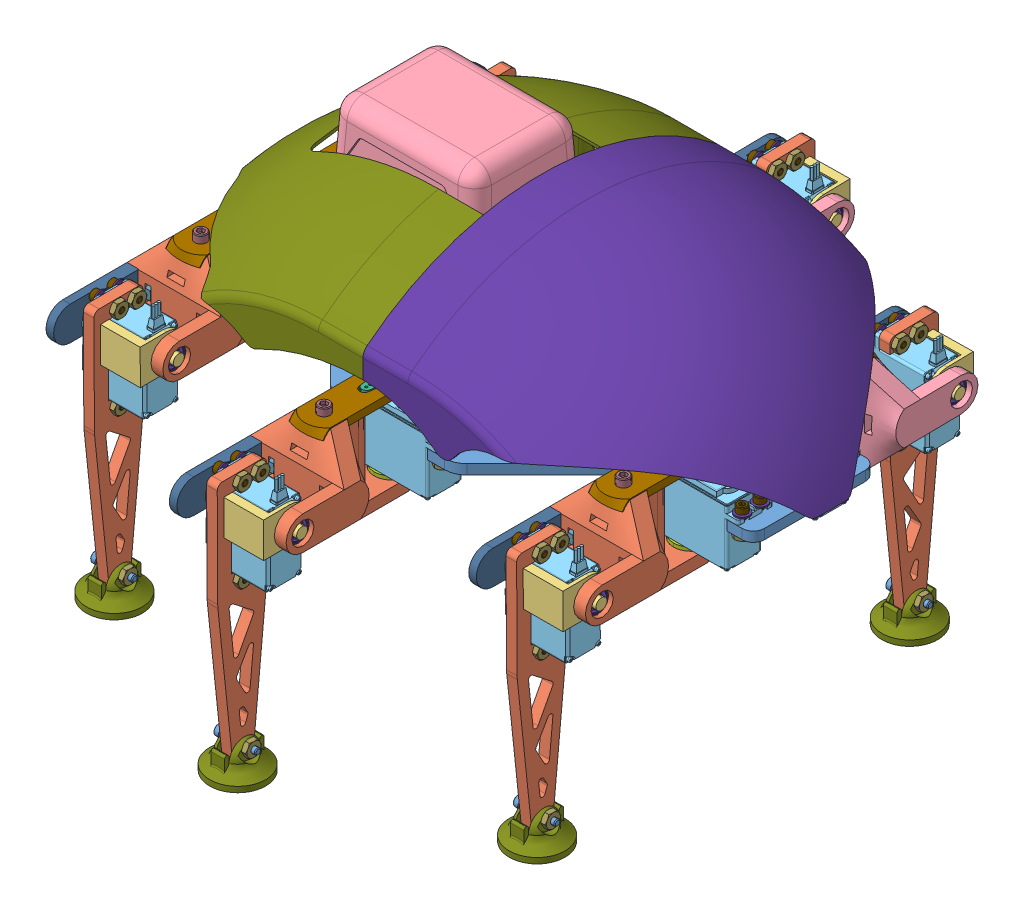
SolidWorks assembly Hexapod, configuration Défaut. Lengths in mm. (continued)
Components (placement in the parent): (continued)
- Leg_(Straight_Foot)_(Mirror)-5: Leg_(Straight_Foot)_(Mirror) [Default] at (-54.94 -26.67 49.906) size (70.36 162.3 124.8) (flexible) (continued)
  - HX-SHCS 0.138-32x0.5x0.5-N-15: HX-SHCS 0.138-32x0.5x0.5-N [HX-SHCS 0.138-32x0.5x0.5-N] at (-7.0087 -17.0352 62.351) x (0.999998 0 -0.002055) z (0.002055 0 0.999998) size (16.21 5.74 5.74)
  - HX-SHCS 0.138-32x0.5x0.5-N-16: HX-SHCS 0.138-32x0.5x0.5-N [HX-SHCS 0.138-32x0.5x0.5-N] at (-6.9874 30.4142 72.7445) x (0.999998 0 -0.002055) z (0.002055 0 0.999998) size (16.21 5.74 5.74)
  - HX-SHCS 0.138-32x0.5x0.5-N-17: HX-SHCS 0.138-32x0.5x0.5-N [HX-SHCS 0.138-32x0.5x0.5-N] at (-6.9878 -17.0852 72.5109) x (0.999998 0 -0.002055) z (0.002055 0 0.999998) size (16.21 5.74 5.74)
  - Narrow FW 0.138-8: Narrow FW 0.138 [Narrow FW 0.138] at (-3.81 29.1846 -4.826) x (0 -1 0) z (0.55878 0 -0.829316) size (0.81 7.92 7.92)
  - HX-SHCS 0.138-32x0.5x0.5-N-18: HX-SHCS 0.138-32x0.5x0.5-N [HX-SHCS 0.138-32x0.5x0.5-N] at (-3.81 33.7566 -4.826) x (0 -1 0) z (-0.55878 0 0.829316) size (16.21 5.74 5.74)
  - Narrow FW 0.138-9: Narrow FW 0.138 [Narrow FW 0.138] at (43.69 29.1846 -4.826) x (0 -1 0) z (0.55878 0 -0.829316) size (0.81 7.92 7.92)
  - Narrow FW 0.138-10: Narrow FW 0.138 [Narrow FW 0.138] at (-3.81 29.1846 -14.986) x (0 -1 0) z (0.55878 0 -0.829316) size (0.81 7.92 7.92)
  - Narrow FW 0.138-11: Narrow FW 0.138 [Narrow FW 0.138] at (43.69 29.1846 -14.986) x (0 -1 0) z (0.55878 0 -0.829316) size (0.81 7.92 7.92)
  - HX-SHCS 0.138-32x0.5x0.5-N-19: HX-SHCS 0.138-32x0.5x0.5-N [HX-SHCS 0.138-32x0.5x0.5-N] at (43.69 33.7566 -4.826) x (0 -1 0) z (-0.55878 0 0.829316) size (16.21 5.74 5.74)
  - HX-SHCS 0.138-32x0.5x0.5-N-20: HX-SHCS 0.138-32x0.5x0.5-N [HX-SHCS 0.138-32x0.5x0.5-N] at (-3.81 33.7566 -14.986) x (0 -1 0) z (-0.55878 0 0.829316) size (16.21 5.74 5.74)
  - HX-SHCS 0.138-32x0.5x0.5-N-21: HX-SHCS 0.138-32x0.5x0.5-N [HX-SHCS 0.138-32x0.5x0.5-N] at (43.69 33.7566 -14.986) x (0 -1 0) z (-0.55878 0 0.829316) size (16.21 5.74 5.74)
  - HX-SHCS 0.138-32x0.75x0.75-N-1: HX-SHCS 0.138-32x0.75x0.75-N [HX-SHCS 0.138-32x0.75x0.75-N] at (-7.8263 -99.7276 71.0261) x (0.999998 0 -0.002055) z (-0.001815 -0.46966 -0.882845) size (22.56 5.74 5.74)
  - Narrow FW 0.138-12: Narrow FW 0.138 [Narrow FW 0.138] at (-4.0671 -99.7276 71.0183) x (-0.999998 0 0.002055) z (-0.001688 -0.570502 -0.821294) size (0.81 7.92 7.92)
  - MSHXNUT 0.138-32-D-N-18: MSHXNUT 0.138-32-D-N [MSHXNUT 0.138-32-D-N] at (9.4457 -99.7276 70.9906) x (0 1 0) z (-0.999998 0 0.002055) size (7.92 9.15 2.9)
- Leg_(Straight_Foot)_(Mirror)-6: Leg_(Straight_Foot)_(Mirror) [Default] at (-174.94 -26.67 99.906) size (70.36 162.3 124.8) (flexible)
  - Joint_(Mirror)-1: Joint_(Mirror) [Défaut] at (36.4933 -51.1276 34.4889) x (0.002055 0 0.999998) z (0 -1 0) size (96.52 53.26 53.26)
  - hs-422-3: hs-422 [Défaut] at (19.939 20.701 -19.812) x (0 0 1) z (-1 0 0) size (19.81 42.09 58.23)
  - hs-422_horn_straight-2: hs-422_horn_straight [Default] at (9.652 42.5743 -9.906) x (0.002055 0 0.999998) z (0.999998 0 -0.002055) size (33.93 4.93 8.79)
  - Bearing_mount_leg-1: Bearing_mount_leg [Default] at (9.652 21 -22.406) x (0 0 -1) z (0 -1 0) size (35 20 30)
  - Bearing-1: Bearing [Default] at (9.652 -6.7498 -9.906) x (0.266287 0 0.963894) z (-0.963894 0 0.266287) size (13.87 4.75 13.87)
  - Joint_attachment_leg-1: Joint_attachment_leg [Défaut] at (-17.0066 26.5024 34.5989) x (0.002055 0 0.999998) z (0 1 0) size (74.32 19.07 4.32)
  - bearing_mount_foot-2: bearing_mount_foot [Default] at (6.7141 17.2663 79.9818) x (0.002055 -0.004919 0.999986) z (0.999998 0 -0.002055) size (25 20 29.5)
  - Bearing-3: Bearing [Default] at (29.1886 16.9774 67.524) x (-0.001098 -0.845349 -0.534213) z (0.001738 -0.534214 0.845347) size (13.87 4.75 13.87)
  - hs-422-4: hs-422 [Défaut] at (6.0779 6.6418 77.4268) x (-0.002055 0.004919 -0.999986) z (0.00001 0.999988 0.004919) size (19.81 42.09 58.23)
  - hs-422_horn_straight-3: hs-422_horn_straight [Default] at (-15.8156 16.9774 67.6165) x (-0.002055 0 -0.999998) z (0 -1 0) size (33.93 4.93 8.79)
  - Foot_(Straight)-2: Foot_(Straight) [Default] at (0.0967 4.6719 71.5233) x (-0.002055 0.004919 -0.999986) z (0.999998 0 -0.002055) size (28 145.4 6)
  - Joint_attachment_foot-2: Joint_attachment_foot [Défaut] at (36.4933 7.4524 34.4889) x (0.002055 0 0.999998) z (0 -1 0) size (64.08 6.7 19.07)
  - SBHCSCREW 0.138-32x0.25-HX-N-1: SBHCSCREW 0.138-32x0.25-HX-N [SBHCSCREW 0.138-32x0.25-HX-N] at (-19.1684 16.9774 67.6234) x (0.999998 0 -0.002055) z (0.002055 0 0.999998) size (8.2 6.65 6.65)
  - SBHCSCREW 0.138-32x0.25-HX-N-2: SBHCSCREW 0.138-32x0.25-HX-N [SBHCSCREW 0.138-32x0.25-HX-N] at (9.652 45.9271 -9.906) x (0 -1 0) z (-0.864996 0 0.501779) size (8.2 6.65 6.65)
  - HX-SHCS 0.112-40x0.5x0.5-N-5: HX-SHCS 0.112-40x0.5x0.5-N [HX-SHCS 0.112-40x0.5x0.5-N] at (-2.7306 21.6303 80.0227) x (0.999998 0 -0.002055) z (0.001019 -0.868474 0.495733) size (15.54 4.65 4.65)
  - HX-SHCS 0.112-40x0.5x0.5-N-6: HX-SHCS 0.112-40x0.5x0.5-N [HX-SHCS 0.112-40x0.5x0.5-N] at (-2.7307 11.6304 79.9735) x (0.999998 0 -0.002055) z (0.001036 0.863555 0.504253) size (15.54 4.65 4.65)
  - HX-SHCS 0.164-32x0.5x0.5-N-3: HX-SHCS 0.164-32x0.5x0.5-N [HX-SHCS 0.164-32x0.5x0.5-N] at (-21.1613 16.9774 39.9006) x (0.999998 0 -0.002055) z (0.001028 0.866025 0.499999) size (16.87 6.86 6.86)
  - HX-SHCS 0.164-32x0.5x0.5-N-4: HX-SHCS 0.164-32x0.5x0.5-N [HX-SHCS 0.164-32x0.5x0.5-N] at (9.7311 47.893 28.5918) x (0 -1 0) z (0.002055 0 0.999998) size (16.87 6.86 6.86)
  - MSHXNUT 0.138-32-D-N-14: MSHXNUT 0.138-32-D-N [MSHXNUT 0.138-32-D-N] at (6.0779 -17.0332 62.3241) x (-0.001785 -0.495734 -0.868473) z (-0.999998 0 0.002055) size (7.92 9.15 2.9)
  - MSHXNUT 0.138-32-D-N-15: MSHXNUT 0.138-32-D-N [MSHXNUT 0.138-32-D-N] at (8.9943 -17.0832 72.478) x (-0.001775 0.504254 -0.863554) z (0.999998 0 -0.002055) size (7.92 9.15 2.9)
  - MSHXNUT 0.138-32-D-N-16: MSHXNUT 0.138-32-D-N [MSHXNUT 0.138-32-D-N] at (8.9739 30.4662 62.5518) x (0.00001 0.999988 0.004919) z (0.999998 0 -0.002055) size (7.92 9.15 2.9)
  - MSHXNUT 0.138-32-D-N-17: MSHXNUT 0.138-32-D-N [MSHXNUT 0.138-32-D-N] at (6.0992 30.4162 72.7176) x (-0.001785 -0.495734 -0.868473) z (-0.999998 0 0.002055) size (7.92 9.15 2.9)
  - MSHXNUT 0.164-32-D-N-10: MSHXNUT 0.164-32-D-N [MSHXNUT 0.164-32-D-N] at (-6.4315 16.9774 39.8703) x (0.002055 0 0.999998) z (-0.999998 0 0.002055) size (8.74 10.09 3.3)
  - MSHXNUT 0.164-32-D-N-11: MSHXNUT 0.164-32-D-N [MSHXNUT 0.164-32-D-N] at (9.7311 29.8612 28.5918) x (-0.002055 0 -0.999998) z (0 -1 0) size (8.74 10.09 3.3)
  - Slipper-1: Slipper [Default] at (3.0957 -111.2276 71.0036) x (0.999998 0 -0.002055) z (0.002055 0 0.999998) size (35.48 18.25 37.71)
  - Narrow FW 0.138-4: Narrow FW 0.138 [Narrow FW 0.138] at (-2.4363 30.4642 62.5753) x (0.999998 0 -0.002055) z (0.002055 0 0.999998) size (0.81 7.92 7.92)
  - HX-SHCS 0.138-32x0.5x0.5-N-14: HX-SHCS 0.138-32x0.5x0.5-N [HX-SHCS 0.138-32x0.5x0.5-N] at (-7.0082 30.4642 62.5847) x (0.999998 0 -0.002055) z (0.002055 0 0.999998) size (16.21 5.74 5.74)
  - Narrow FW 0.138-5: Narrow FW 0.138 [Narrow FW 0.138] at (-2.4367 -17.0352 62.3416) x (0.999998 0 -0.002055) z (0.002055 0 0.999998) size (0.81 7.92 7.92)
  - Narrow FW 0.138-6: Narrow FW 0.138 [Narrow FW 0.138] at (-2.4154 30.4142 72.7351) x (0.999998 0 -0.002055) z (0.002055 0 0.999998) size (0.81 7.92 7.92)
  - Narrow FW 0.138-7: Narrow FW 0.138 [Narrow FW 0.138] at (-2.4158 -17.0852 72.5015) x (0.999998 0 -0.002055) z (0.002055 0 0.999998) size (0.81 7.92 7.92)
  - HX-SHCS 0.138-32x0.5x0.5-N-15: HX-SHCS 0.138-32x0.5x0.5-N [HX-SHCS 0.138-32x0.5x0.5-N] at (-7.0087 -17.0352 62.351) x (0.999998 0 -0.002055) z (0.002055 0 0.999998) size (16.21 5.74 5.74)
  - HX-SHCS 0.138-32x0.5x0.5-N-16: HX-SHCS 0.138-32x0.5x0.5-N [HX-SHCS 0.138-32x0.5x0.5-N] at (-6.9874 30.4142 72.7445) x (0.999998 0 -0.002055) z (0.002055 0 0.999998) size (16.21 5.74 5.74)
  - HX-SHCS 0.138-32x0.5x0.5-N-17: HX-SHCS 0.138-32x0.5x0.5-N [HX-SHCS 0.138-32x0.5x0.5-N] at (-6.9878 -17.0852 72.5109) x (0.999998 0 -0.002055) z (0.002055 0 0.999998) size (16.21 5.74 5.74)
  - Narrow FW 0.138-8: Narrow FW 0.138 [Narrow FW 0.138] at (-3.81 29.1846 -4.826) x (0 -1 0) z (0.55878 0 -0.829316) size (0.81 7.92 7.92)
  - HX-SHCS 0.138-32x0.5x0.5-N-18: HX-SHCS 0.138-32x0.5x0.5-N [HX-SHCS 0.138-32x0.5x0.5-N] at (-3.81 33.7566 -4.826) x (0 -1 0) z (-0.55878 0 0.829316) size (16.21 5.74 5.74)
  - Narrow FW 0.138-9: Narrow FW 0.138 [Narrow FW 0.138] at (43.69 29.1846 -4.826) x (0 -1 0) z (0.55878 0 -0.829316) size (0.81 7.92 7.92)
  - Narrow FW 0.138-10: Narrow FW 0.138 [Narrow FW 0.138] at (-3.81 29.1846 -14.986) x (0 -1 0) z (0.55878 0 -0.829316) size (0.81 7.92 7.92)
  - Narrow FW 0.138-11: Narrow FW 0.138 [Narrow FW 0.138] at (43.69 29.1846 -14.986) x (0 -1 0) z (0.55878 0 -0.829316) size (0.81 7.92 7.92)
  - HX-SHCS 0.138-32x0.5x0.5-N-19: HX-SHCS 0.138-32x0.5x0.5-N [HX-SHCS 0.138-32x0.5x0.5-N] at (43.69 33.7566 -4.826) x (0 -1 0) z (-0.55878 0 0.829316) size (16.21 5.74 5.74)
  - HX-SHCS 0.138-32x0.5x0.5-N-20: HX-SHCS 0.138-32x0.5x0.5-N [HX-SHCS 0.138-32x0.5x0.5-N] at (-3.81 33.7566 -14.986) x (0 -1 0) z (-0.55878 0 0.829316) size (16.21 5.74 5.74)
  - HX-SHCS 0.138-32x0.5x0.5-N-21: HX-SHCS 0.138-32x0.5x0.5-N [HX-SHCS 0.138-32x0.5x0.5-N] at (43.69 33.7566 -14.986) x (0 -1 0) z (-0.55878 0 0.829316) size (16.21 5.74 5.74)
  - HX-SHCS 0.138-32x0.75x0.75-N-1: HX-SHCS 0.138-32x0.75x0.75-N [HX-SHCS 0.138-32x0.75x0.75-N] at (-7.8263 -99.7276 71.0261) x (0.999998 0 -0.002055) z (-0.001815 -0.46966 -0.882845) size (22.56 5.74 5.74)
  - Narrow FW 0.138-12: Narrow FW 0.138 [Narrow FW 0.138] at (-4.0671 -99.7276 71.0183) x (-0.999998 0 0.002055) z (-0.001688 -0.570502 -0.821294) size (0.81 7.92 7.92)
  - MSHXNUT 0.138-32-D-N-18: MSHXNUT 0.138-32-D-N [MSHXNUT 0.138-32-D-N] at (9.4457 -99.7276 70.9906) x (0 1 0) z (-0.999998 0 0.002055) size (7.92 9.15 2.9)
- Battery-1: Battery [Défaut] at (-118.1821 62.8376 15.5603) x (0 0 -1) z (-1 0 0) size (64.47 74.3 85.78)
  - MAKITA 4.0AH-1: MAKITA 4.0AH [Défaut] at (0.5853 -29.7874 85.4436) size (64.47 57.15 85.78)
  - MAKITA 4.0AH MOBILE-1: MAKITA 4.0AH MOBILE [Défaut] at (0.5853 -39.3124 91.7936) size (45.84 26.68 66.29)
- arduinoMega-1: arduinoMega [Detailed] at (-199.11 -7.6 14.62) x (0 0 -1) z (-1 0 0) size (108.32 14.5 53.3)
- raspberryPi3B-1: raspberryPi3B [Detailed] at (-109 6.35 15) x (-1 0 0) z (0 1 0) size (87.05 58.5 19.5)
- 12Channel PWM-1: 12Channel PWM [Default] at (-145.6 -5.6 15) x (-1 0 0) z (0 0 1) size (25.4 7.55 66.7)
- DROK_090483.stp-1: DROK_090483.stp [Default] at (-77.5 -5.6 45) x (-1 0 0) z (0 -1 0) size (50.02 60 18.9)
- HX-SHCS 0.138-32x0.625x0.625-N-2: HX-SHCS 0.138-32x0.625x0.625-N [HX-SHCS 0.138-32x0.625x0.625-N] at (-40.288 3.5052 19.09) x (0 -1 0) z (1 0 0) size (19.38 5.74 5.74)
- HX-SHCS 0.138-32x0.625x0.625-N-3: HX-SHCS 0.138-32x0.625x0.625-N [HX-SHCS 0.138-32x0.625x0.625-N] at (-50.288 3.5052 19.09) x (0 -1 0) z (0.5 0 0.866025) size (19.38 5.74 5.74)
- HX-SHCS 0.138-32x0.625x0.625-N-4: HX-SHCS 0.138-32x0.625x0.625-N [HX-SHCS 0.138-32x0.625x0.625-N] at (-50.288 3.5052 10.91) x (0 -1 0) z (1 0 0) size (19.38 5.74 5.74)
- HX-SHCS 0.138-32x0.625x0.625-N-5: HX-SHCS 0.138-32x0.625x0.625-N [HX-SHCS 0.138-32x0.625x0.625-N] at (-40.288 3.5052 10.91) x (0 -1 0) z (1 0 0) size (19.38 5.74 5.74)
- HX-SHCS 0.138-32x0.625x0.625-N-6: HX-SHCS 0.138-32x0.625x0.625-N [HX-SHCS 0.138-32x0.625x0.625-N] at (-170.288 3.5052 69.09) x (0 -1 0) z (1 0 0) size (19.38 5.74 5.74)
- HX-SHCS 0.138-32x0.625x0.625-N-7: HX-SHCS 0.138-32x0.625x0.625-N [HX-SHCS 0.138-32x0.625x0.625-N] at (-160.288 3.5052 69.09) x (0 -1 0) z (1 0 0) size (19.38 5.74 5.74)
- HX-SHCS 0.138-32x0.625x0.625-N-14: HX-SHCS 0.138-32x0.625x0.625-N [HX-SHCS 0.138-32x0.625x0.625-N] at (-160.288 3.5052 -39.09) x (0 -1 0) z (1 0 0) size (19.38 5.74 5.74)
- HX-SHCS 0.138-32x0.625x0.625-N-15: HX-SHCS 0.138-32x0.625x0.625-N [HX-SHCS 0.138-32x0.625x0.625-N] at (-170.288 3.5052 -39.09) x (0 -1 0) z (1 0 0) size (19.38 5.74 5.74)
- HX-SHCS 0.138-32x0.625x0.625-N-16: HX-SHCS 0.138-32x0.625x0.625-N [HX-SHCS 0.138-32x0.625x0.625-N] at (-280.288 3.5052 19.09) x (0 -1 0) z (1 0 0) size (19.38 5.74 5.74)
- HX-SHCS 0.138-32x0.625x0.625-N-17: HX-SHCS 0.138-32x0.625x0.625-N [HX-SHCS 0.138-32x0.625x0.625-N] at (-290.288 3.5052 19.09) x (0 -1 0) z (0.5 0 0.866025) size (19.38 5.74 5.74)
- HX-SHCS 0.138-32x0.625x0.625-N-18: HX-SHCS 0.138-32x0.625x0.625-N [HX-SHCS 0.138-32x0.625x0.625-N] at (-290.288 3.5052 10.91) x (0 -1 0) z (1 0 0) size (19.38 5.74 5.74)
- HX-SHCS 0.138-32x0.625x0.625-N-19: HX-SHCS 0.138-32x0.625x0.625-N [HX-SHCS 0.138-32x0.625x0.625-N] at (-280.288 3.5052 10.91) x (0 -1 0) z (1 0 0) size (19.38 5.74 5.74)
- MSHXNUT 0.138-32-D-N-60: MSHXNUT 0.138-32-D-N [MSHXNUT 0.138-32-D-N] at (-298.75 -8.4956 -15.08) x (1 0 0) z (0 -1 0) size (7.92 9.15 2.9)
- MSHXNUT 0.138-32-D-N-65: MSHXNUT 0.138-32-D-N [MSHXNUT 0.138-32-D-N] at (-298.75 -8.4956 -4.92) x (1 0 0) z (0 -1 0) size (7.92 9.15 2.9)
- MSHXNUT 0.138-32-D-N-70: MSHXNUT 0.138-32-D-N [MSHXNUT 0.138-32-D-N] at (-251.252 -8.4956 -4.92) x (0.5 0 0.866025) z (0 -1 0) size (7.92 9.15 2.9)
- MSHXNUT 0.138-32-D-N-75: MSHXNUT 0.138-32-D-N [MSHXNUT 0.138-32-D-N] at (-251.252 -8.4956 -15.08) x (0.5 0 0.866025) z (0 -1 0) size (7.92 9.15 2.9)
- MSHXNUT 0.138-32-D-N-80: MSHXNUT 0.138-32-D-N [MSHXNUT 0.138-32-D-N] at (-280.288 -13.5656 10.91) x (0 0 1) z (0 -1 0) size (7.92 9.15 2.9)
- MSHXNUT 0.138-32-D-N-85: MSHXNUT 0.138-32-D-N [MSHXNUT 0.138-32-D-N] at (-290.288 -13.5656 10.91) x (0 0 1) z (0 -1 0) size (7.92 9.15 2.9)
- MSHXNUT 0.138-32-D-N-88: MSHXNUT 0.138-32-D-N [MSHXNUT 0.138-32-D-N] at (-178.75 -8.4956 -65.08) x (1 0 0) z (0 -1 0) size (7.92 9.15 2.9)
- MSHXNUT 0.138-32-D-N-89: MSHXNUT 0.138-32-D-N [MSHXNUT 0.138-32-D-N] at (-178.75 -8.4956 -54.92) x (1 0 0) z (0 -1 0) size (7.92 9.15 2.9)
- MSHXNUT 0.138-32-D-N-90: MSHXNUT 0.138-32-D-N [MSHXNUT 0.138-32-D-N] at (-131.252 -8.4956 -54.92) x (0.5 0 0.866025) z (0 -1 0) size (7.92 9.15 2.9)
- MSHXNUT 0.138-32-D-N-91: MSHXNUT 0.138-32-D-N [MSHXNUT 0.138-32-D-N] at (-131.252 -8.4956 -65.08) x (0.5 0 0.866025) z (0 -1 0) size (7.92 9.15 2.9)
- MSHXNUT 0.138-32-D-N-92: MSHXNUT 0.138-32-D-N [MSHXNUT 0.138-32-D-N] at (-160.288 -13.5656 -39.09) x (0 0 1) z (0 -1 0) size (7.92 9.15 2.9)
- MSHXNUT 0.138-32-D-N-93: MSHXNUT 0.138-32-D-N [MSHXNUT 0.138-32-D-N] at (-170.288 -13.5656 -39.09) x (0 0 1) z (0 -1 0) size (7.92 9.15 2.9)
- MSHXNUT 0.138-32-D-N-94: MSHXNUT 0.138-32-D-N [MSHXNUT 0.138-32-D-N] at (-50.288 -13.5656 10.91) x (0 0 1) z (0 -1 0) size (7.92 9.15 2.9)
- MSHXNUT 0.138-32-D-N-95: MSHXNUT 0.138-32-D-N [MSHXNUT 0.138-32-D-N] at (-40.288 -13.5656 10.91) x (0 0 1) z (0 -1 0) size (7.92 9.15 2.9)
- MSHXNUT 0.138-32-D-N-96: MSHXNUT 0.138-32-D-N [MSHXNUT 0.138-32-D-N] at (-11.252 -8.4956 -4.92) x (0.5 0 0.866025) z (0 -1 0) size (7.92 9.15 2.9)
- MSHXNUT 0.138-32-D-N-97: MSHXNUT 0.138-32-D-N [MSHXNUT 0.138-32-D-N] at (-11.252 -8.4956 -15.08) x (0.5 0 0.866025) z (0 -1 0) size (7.92 9.15 2.9)
- MSHXNUT 0.138-32-D-N-98: MSHXNUT 0.138-32-D-N [MSHXNUT 0.138-32-D-N] at (-58.75 -8.4956 -4.92) x (1 0 0) z (0 -1 0) size (7.92 9.15 2.9)
- MSHXNUT 0.138-32-D-N-99: MSHXNUT 0.138-32-D-N [MSHXNUT 0.138-32-D-N] at (-58.75 -8.4956 -15.08) x (1 0 0) z (0 -1 0) size (7.92 9.15 2.9)
- MSHXNUT 0.138-32-D-N-100: MSHXNUT 0.138-32-D-N [MSHXNUT 0.138-32-D-N] at (-290.288 -10.67 19.09) x (0 0 -1) z (0 1 0) size (7.92 9.15 2.9)
- MSHXNUT 0.138-32-D-N-101: MSHXNUT 0.138-32-D-N [MSHXNUT 0.138-32-D-N] at (-280.288 -10.67 19.09) x (0 0 -1) z (0 1 0) size (7.92 9.15 2.9)
- MSHXNUT 0.138-32-D-N-102: MSHXNUT 0.138-32-D-N [MSHXNUT 0.138-32-D-N] at (-251.252 -5.6 34.92) x (0.5 0 -0.866025) z (0 1 0) size (7.92 9.15 2.9)
- MSHXNUT 0.138-32-D-N-103: MSHXNUT 0.138-32-D-N [MSHXNUT 0.138-32-D-N] at (-251.252 -5.6 45.08) x (0.5 0 -0.866025) z (0 1 0) size (7.92 9.15 2.9)
- MSHXNUT 0.138-32-D-N-104: MSHXNUT 0.138-32-D-N [MSHXNUT 0.138-32-D-N] at (-298.75 -5.6 34.92) x (1 0 0) z (0 1 0) size (7.92 9.15 2.9)
- MSHXNUT 0.138-32-D-N-105: MSHXNUT 0.138-32-D-N [MSHXNUT 0.138-32-D-N] at (-298.75 -5.6 45.08) x (1 0 0) z (0 1 0) size (7.92 9.15 2.9)
- MSHXNUT 0.138-32-D-N-106: MSHXNUT 0.138-32-D-N [MSHXNUT 0.138-32-D-N] at (-178.75 -5.6 95.08) x (1 0 0) z (0 1 0) size (7.92 9.15 2.9)
- MSHXNUT 0.138-32-D-N-107: MSHXNUT 0.138-32-D-N [MSHXNUT 0.138-32-D-N] at (-178.75 -5.6 84.92) x (1 0 0) z (0 1 0) size (7.92 9.15 2.9)
- MSHXNUT 0.138-32-D-N-108: MSHXNUT 0.138-32-D-N [MSHXNUT 0.138-32-D-N] at (-131.252 -5.6 84.92) x (0.5 0 -0.866025) z (0 1 0) size (7.92 9.15 2.9)
- MSHXNUT 0.138-32-D-N-109: MSHXNUT 0.138-32-D-N [MSHXNUT 0.138-32-D-N] at (-131.252 -5.6 95.08) x (0.5 0 -0.866025) z (0 1 0) size (7.92 9.15 2.9)
- MSHXNUT 0.138-32-D-N-110: MSHXNUT 0.138-32-D-N [MSHXNUT 0.138-32-D-N] at (-160.288 -10.67 69.09) x (0 0 -1) z (0 1 0) size (7.92 9.15 2.9)
- MSHXNUT 0.138-32-D-N-111: MSHXNUT 0.138-32-D-N [MSHXNUT 0.138-32-D-N] at (-170.288 -10.67 69.09) x (0 0 -1) z (0 1 0) size (7.92 9.15 2.9)
- MSHXNUT 0.138-32-D-N-112: MSHXNUT 0.138-32-D-N [MSHXNUT 0.138-32-D-N] at (-50.288 -10.67 19.09) x (0 0 -1) z (0 1 0) size (7.92 9.15 2.9)
- MSHXNUT 0.138-32-D-N-113: MSHXNUT 0.138-32-D-N [MSHXNUT 0.138-32-D-N] at (-40.288 -10.67 19.09) x (0 0 -1) z (0 1 0) size (7.92 9.15 2.9)
- MSHXNUT 0.138-32-D-N-114: MSHXNUT 0.138-32-D-N [MSHXNUT 0.138-32-D-N] at (-11.252 -5.6 34.92) x (0.5 0 -0.866025) z (0 1 0) size (7.92 9.15 2.9)
- MSHXNUT 0.138-32-D-N-115: MSHXNUT 0.138-32-D-N [MSHXNUT 0.138-32-D-N] at (-11.252 -5.6 45.08) x (0.5 0 -0.866025) z (0 1 0) size (7.92 9.15 2.9)
- MSHXNUT 0.138-32-D-N-116: MSHXNUT 0.138-32-D-N [MSHXNUT 0.138-32-D-N] at (-58.75 -5.6 34.92) x (1 0 0) z (0 1 0) size (7.92 9.15 2.9)
- MSHXNUT 0.138-32-D-N-117: MSHXNUT 0.138-32-D-N [MSHXNUT 0.138-32-D-N] at (-58.75 -5.6 45.08) x (1 0 0) z (0 1 0) size (7.92 9.15 2.9)
- HX-SHCS 0.138-32x0.5x0.5-N-20: HX-SHCS 0.138-32x0.5x0.5-N [HX-SHCS 0.138-32x0.5x0.5-N] at (-175 -12.6052 48.88) x (0 1 0) z (-0.5 0 -0.866025) size (16.21 5.74 5.74)
- HX-SHCS 0.138-32x0.5x0.5-N-21: HX-SHCS 0.138-32x0.5x0.5-N [HX-SHCS 0.138-32x0.5x0.5-N] at (-223.22 -12.6052 -32.36) x (0 1 0) z (1 0 0) size (16.21 5.74 5.74)
- HX-SHCS 0.138-32x0.5x0.5-N-22: HX-SHCS 0.138-32x0.5x0.5-N [HX-SHCS 0.138-32x0.5x0.5-N] at (-175 -12.6052 -26) x (0 1 0) z (-0.5 0 -0.866025) size (16.21 5.74 5.74)
- HX-SHCS 0.138-32x0.5x0.5-N-23: HX-SHCS 0.138-32x0.5x0.5-N [HX-SHCS 0.138-32x0.5x0.5-N] at (-223.22 -12.6052 50.11) x (0 1 0) z (-1 0 0) size (16.21 5.74 5.74)
- MSHXNUT 0.112-40-D-N-106: MSHXNUT 0.112-40-D-N [MSHXNUT 0.112-40-D-N] at (-223.22 2.4892 -32.36) x (1 0 0) z (0 1 0) size (6.35 7.33 2.49)
- MSHXNUT 0.112-40-D-N-107: MSHXNUT 0.112-40-D-N [MSHXNUT 0.112-40-D-N] at (-223.22 2.4892 50.11) x (1 0 0) z (0 1 0) size (6.35 7.33 2.49)
- MSHXNUT 0.112-40-D-N-108: MSHXNUT 0.112-40-D-N [MSHXNUT 0.112-40-D-N] at (-175 2.4892 -26) x (1 0 0) z (0 1 0) size (6.35 7.33 2.49)
- MSHXNUT 0.112-40-D-N-109: MSHXNUT 0.112-40-D-N [MSHXNUT 0.112-40-D-N] at (-175 2.4892 48.88) x (1 0 0) z (0 1 0) size (6.35 7.33 2.49)
- HX-SHCS 0.138-32x0.5x0.5-N-24: HX-SHCS 0.138-32x0.5x0.5-N [HX-SHCS 0.138-32x0.5x0.5-N] at (-117.315 -10.3052 -11.415) x (0 1 0) z (-0.5 0 -0.866025) size (16.21 5.74 5.74)
- MSHXNUT 0.112-40-D-N-110: MSHXNUT 0.112-40-D-N [MSHXNUT 0.112-40-D-N] at (-117.315 2.4892 -11.415) x (1 0 0) z (0 1 0) size (6.35 7.33 2.49)
- HX-SHCS 0.138-32x0.5x0.5-N-28: HX-SHCS 0.138-32x0.5x0.5-N [HX-SHCS 0.138-32x0.5x0.5-N] at (-80.685 -10.3052 -11.415) x (0 1 0) z (-0.5 0 -0.866025) size (16.21 5.74 5.74)
- HX-SHCS 0.138-32x0.5x0.5-N-29: HX-SHCS 0.138-32x0.5x0.5-N [HX-SHCS 0.138-32x0.5x0.5-N] at (-117.315 -10.3052 41.415) x (0 1 0) z (-0.5 0 -0.866025) size (16.21 5.74 5.74)
- HX-SHCS 0.138-32x0.5x0.5-N-30: HX-SHCS 0.138-32x0.5x0.5-N [HX-SHCS 0.138-32x0.5x0.5-N] at (-80.685 -10.3052 41.415) x (0 1 0) z (-0.5 0 -0.866025) size (16.21 5.74 5.74)
- MSHXNUT 0.112-40-D-N-114: MSHXNUT 0.112-40-D-N [MSHXNUT 0.112-40-D-N] at (-80.685 2.4892 -11.415) x (1 0 0) z (0 1 0) size (6.35 7.33 2.49)
- MSHXNUT 0.112-40-D-N-115: MSHXNUT 0.112-40-D-N [MSHXNUT 0.112-40-D-N] at (-117.315 2.4892 41.415) x (1 0 0) z (0 1 0) size (6.35 7.33 2.49)
- MSHXNUT 0.112-40-D-N-116: MSHXNUT 0.112-40-D-N [MSHXNUT 0.112-40-D-N] at (-80.685 2.4892 41.415) x (1 0 0) z (0 1 0) size (6.35 7.33 2.49)
- 1_4_Round_Aluminum_Standoff.step-1: 1_4_Round_Aluminum_Standoff.step [Défaut] at (-70 0 -9.5) x (0.963282 0 -0.268492) z (0.268492 0 0.963282) size (6.34 6.36 6.34)
- HX-SHCS 0.112-40x0.75x0.75-N-65: HX-SHCS 0.112-40x0.75x0.75-N [HX-SHCS 0.112-40x0.75x0.75-N] at (-70 10.4948 -9.5) x (0 -1 0) z (0.637638 0 0.770336) size (21.89 4.65 4.65)
- MSHXNUT 0.112-40-D-N-117: MSHXNUT 0.112-40-D-N [MSHXNUT 0.112-40-D-N] at (-70 -8.0892 -9.5) x (1 0 0) z (0 -1 0) size (6.35 7.33 2.49)
- 1_4_Round_Aluminum_Standoff.step-2: 1_4_Round_Aluminum_Standoff.step [Défaut] at (-128 0 -9.5) x (0.963282 0 -0.268492) z (0.268492 0 0.963282) size (6.34 6.36 6.34)
- 1_4_Round_Aluminum_Standoff.step-3: 1_4_Round_Aluminum_Standoff.step [Défaut] at (-70 0 39.5) x (0.963282 0 -0.268492) z (0.268492 0 0.963282) size (6.34 6.36 6.34)
- 1_4_Round_Aluminum_Standoff.step-4: 1_4_Round_Aluminum_Standoff.step [Défaut] at (-128 0 39.5) x (0.963282 0 -0.268492) z (0.268492 0 0.963282) size (6.34 6.36 6.34)
- MSHXNUT 0.112-40-D-N-121: MSHXNUT 0.112-40-D-N [MSHXNUT 0.112-40-D-N] at (-128 -8.0892 -9.5) x (1 0 0) z (0 -1 0) size (6.35 7.33 2.49)
- MSHXNUT 0.112-40-D-N-122: MSHXNUT 0.112-40-D-N [MSHXNUT 0.112-40-D-N] at (-70 -8.0892 39.5) x (1 0 0) z (0 -1 0) size (6.35 7.33 2.49)
- MSHXNUT 0.112-40-D-N-123: MSHXNUT 0.112-40-D-N [MSHXNUT 0.112-40-D-N] at (-128 -8.0892 39.5) x (1 0 0) z (0 -1 0) size (6.35 7.33 2.49)
- HX-SHCS 0.112-40x0.75x0.75-N-72: HX-SHCS 0.112-40x0.75x0.75-N [PreviewCfg] at (-128 10.4948 -9.5) x (0 -1 0) z (0.637638 0 0.770336) size (28.24 4.65 4.65)
- HX-SHCS 0.112-40x0.75x0.75-N-70: HX-SHCS 0.112-40x0.75x0.75-N [PreviewCfg] at (-70 10.4948 39.5) x (0 -1 0) z (0.637638 0 0.770336) size (28.24 4.65 4.65)
- HX-SHCS 0.112-40x0.75x0.75-N-71: HX-SHCS 0.112-40x0.75x0.75-N [PreviewCfg] at (-128 10.4948 39.5) x (0 -1 0) z (0.637638 0 0.770336) size (28.24 4.65 4.65)
- HX-SHCS 0.112-40x0.5x0.5-N-32: HX-SHCS 0.112-40x0.5x0.5-N [HX-SHCS 0.112-40x0.5x0.5-N] at (-155 -9.9448 -12.95) x (0 1 0) z (-1 0 0) size (15.54 4.65 4.65)
- MSHXNUT 0.112-40-D-N-124: MSHXNUT 0.112-40-D-N [MSHXNUT 0.112-40-D-N] at (-155 2.4892 -12.95) x (1 0 0) z (0 1 0) size (6.35 7.33 2.49)
- HX-SHCS 0.112-40x0.5x0.5-N-36: HX-SHCS 0.112-40x0.5x0.5-N [HX-SHCS 0.112-40x0.5x0.5-N] at (-136.2 -9.9448 -12.95) x (0 1 0) z (-1 0 0) size (15.54 4.65 4.65)
- HX-SHCS 0.112-40x0.5x0.5-N-37: HX-SHCS 0.112-40x0.5x0.5-N [HX-SHCS 0.112-40x0.5x0.5-N] at (-155 -9.9448 42.95) x (0 1 0) z (-1 0 0) size (15.54 4.65 4.65)
- HX-SHCS 0.112-40x0.5x0.5-N-38: HX-SHCS 0.112-40x0.5x0.5-N [HX-SHCS 0.112-40x0.5x0.5-N] at (-136.2 -9.9448 42.95) x (0 1 0) z (-1 0 0) size (15.54 4.65 4.65)
- MSHXNUT 0.112-40-D-N-128: MSHXNUT 0.112-40-D-N [MSHXNUT 0.112-40-D-N] at (-136.2 2.4892 -12.95) x (1 0 0) z (0 1 0) size (6.35 7.33 2.49)
- MSHXNUT 0.112-40-D-N-129: MSHXNUT 0.112-40-D-N [MSHXNUT 0.112-40-D-N] at (-155 2.4892 42.95) x (1 0 0) z (0 1 0) size (6.35 7.33 2.49)
- MSHXNUT 0.112-40-D-N-130: MSHXNUT 0.112-40-D-N [MSHXNUT 0.112-40-D-N] at (-136.2 2.4892 42.95) x (1 0 0) z (0 1 0) size (6.35 7.33 2.49)
- 1_4_Round_Aluminum_Standoff.step-5: 1_4_Round_Aluminum_Standoff.step [Défaut] at (-174 0 -7) x (0.963282 0 -0.268492) z (0.268492 0 0.963282) size (6.34 6.36 6.34)
- 1_4_Round_Aluminum_Standoff.step-6: 1_4_Round_Aluminum_Standoff.step [Défaut] at (-174 0 37) x (0.963282 0 -0.268492) z (0.268492 0 0.963282) size (6.34 6.36 6.34)
- 1_4_Round_Aluminum_Standoff.step-7: 1_4_Round_Aluminum_Standoff.step [Défaut] at (-240 0 -7) x (0.963282 0 -0.268492) z (0.268492 0 0.963282) size (6.34 6.36 6.34)
- 1_4_Round_Aluminum_Standoff.step-8: 1_4_Round_Aluminum_Standoff.step [Défaut] at (-240 0 37) x (0.963282 0 -0.268492) z (0.268492 0 0.963282) size (6.34 6.36 6.34)
- HX-SHCS 0.112-40x1x0.75-N-72: HX-SHCS 0.112-40x1x0.75-N [HX-SHCS 0.112-40x1x0.75-N] at (-174 -8.4448 -7) x (0 1 0) z (-0.415316 0 -0.909677) size (28.24 4.65 4.65)
- HX-SHCS 0.112-40x1x0.75-N-76: HX-SHCS 0.112-40x1x0.75-N [HX-SHCS 0.112-40x1x0.75-N] at (-174 -8.4448 37) x (0 1 0) z (-0.415316 0 -0.909677) size (28.24 4.65 4.65)
- HX-SHCS 0.112-40x1x0.75-N-77: HX-SHCS 0.112-40x1x0.75-N [HX-SHCS 0.112-40x1x0.75-N] at (-240 -8.4448 -7) x (0 1 0) z (-0.415316 0 -0.909677) size (28.24 4.65 4.65)
- HX-SHCS 0.112-40x1x0.75-N-78: HX-SHCS 0.112-40x1x0.75-N [HX-SHCS 0.112-40x1x0.75-N] at (-240 -8.4448 37) x (0 1 0) z (-0.415316 0 -0.909677) size (28.24 4.65 4.65)
- Battery_holder-1: Battery_holder [Default] at (-223 17.7 15) size (72 19.6 50)
- MSHXNUT 0.112-40-D-N-131: MSHXNUT 0.112-40-D-N [MSHXNUT 0.112-40-D-N] at (-174 15.1892 -7) x (1 0 0) z (0 1 0) size (6.35 7.33 2.49)
- MSHXNUT 0.112-40-D-N-135: MSHXNUT 0.112-40-D-N [MSHXNUT 0.112-40-D-N] at (-174 15.1892 37) x (1 0 0) z (0 1 0) size (6.35 7.33 2.49)
- MSHXNUT 0.112-40-D-N-136: MSHXNUT 0.112-40-D-N [MSHXNUT 0.112-40-D-N] at (-240 15.1892 -7) x (1 0 0) z (0 1 0) size (6.35 7.33 2.49)
- MSHXNUT 0.112-40-D-N-137: MSHXNUT 0.112-40-D-N [MSHXNUT 0.112-40-D-N] at (-240 15.1892 37) x (1 0 0) z (0 1 0) size (6.35 7.33 2.49)
- Shell_(Front)-3: Shell_(Front) [Default] at (-155 -76.2 15) x (0 0 1) z (-1 0 0) size (204.71 79.03 165.14)
- Shell_(Back)-3: Shell_(Back) [Default] at (-155 -76.2 15) x (0 0 -1) z (1 0 0) size (205.09 91.22 173.55)
- HX-SHCS 0.138-32x0.625x0.625-N-20: HX-SHCS 0.138-32x0.625x0.625-N [HX-SHCS 0.138-32x0.625x0.625-N] at (-114.1421 9.8552 80) x (0 -1 0) z (-0.546944 0 0.837169) size (19.38 5.74 5.74)
- MSHXNUT 0.138-32-D-N-118: MSHXNUT 0.138-32-D-N [MSHXNUT 0.138-32-D-N] at (-114.1421 -8.4956 80) x (0.5 0 0.866025) z (0 -1 0) size (7.92 9.15 2.9)
- MSHXNUT 0.138-32-D-N-119: MSHXNUT 0.138-32-D-N [MSHXNUT 0.138-32-D-N] at (-96.4645 -8.4956 62.3223) x (0.5 0 0.866025) z (0 -1 0) size (7.92 9.15 2.9)
- HX-SHCS 0.138-32x0.625x0.625-N-21: HX-SHCS 0.138-32x0.625x0.625-N [HX-SHCS 0.138-32x0.625x0.625-N] at (-96.4645 9.8552 62.3223) x (0 -1 0) z (-0.546944 0 0.837169) size (19.38 5.74 5.74)
- MSHXNUT 0.138-32-D-N-120: MSHXNUT 0.138-32-D-N [MSHXNUT 0.138-32-D-N] at (-114.1421 -5.6 -50) x (0.5 0 -0.866025) z (0 1 0) size (7.92 9.15 2.9)
- HX-SHCS 0.138-32x0.625x0.625-N-22: HX-SHCS 0.138-32x0.625x0.625-N [HX-SHCS 0.138-32x0.625x0.625-N] at (-114.1421 9.8552 -50) x (0 -1 0) z (0.546944 0 0.837169) size (19.38 5.74 5.74)
- MSHXNUT 0.138-32-D-N-121: MSHXNUT 0.138-32-D-N [MSHXNUT 0.138-32-D-N] at (-96.4645 -5.6 -32.3223) x (0.5 0 -0.866025) z (0 1 0) size (7.92 9.15 2.9)
- HX-SHCS 0.138-32x0.625x0.625-N-23: HX-SHCS 0.138-32x0.625x0.625-N [HX-SHCS 0.138-32x0.625x0.625-N] at (-96.4645 9.8552 -32.3223) x (0 -1 0) z (0.546944 0 0.837169) size (19.38 5.74 5.74)
- MSHXNUT 0.138-32-D-N-122: MSHXNUT 0.138-32-D-N [MSHXNUT 0.138-32-D-N] at (-195.8579 -5.6 80) x (-0.5 0 0.866025) z (0 1 0) size (7.92 9.15 2.9)
- HX-SHCS 0.138-32x0.625x0.625-N-24: HX-SHCS 0.138-32x0.625x0.625-N [HX-SHCS 0.138-32x0.625x0.625-N] at (-195.8579 9.8552 80) x (0 -1 0) z (-0.546944 0 -0.837169) size (19.38 5.74 5.74)
- MSHXNUT 0.138-32-D-N-123: MSHXNUT 0.138-32-D-N [MSHXNUT 0.138-32-D-N] at (-213.5355 -5.6 62.3223) x (-0.5 0 0.866025) z (0 1 0) size (7.92 9.15 2.9)
- HX-SHCS 0.138-32x0.625x0.625-N-25: HX-SHCS 0.138-32x0.625x0.625-N [HX-SHCS 0.138-32x0.625x0.625-N] at (-213.5355 9.8552 62.3223) x (0 -1 0) z (-0.546944 0 -0.837169) size (19.38 5.74 5.74)
- MSHXNUT 0.138-32-D-N-124: MSHXNUT 0.138-32-D-N [MSHXNUT 0.138-32-D-N] at (-195.8579 -8.4956 -50) x (-0.5 0 -0.866025) z (0 -1 0) size (7.92 9.15 2.9)
- HX-SHCS 0.138-32x0.625x0.625-N-26: HX-SHCS 0.138-32x0.625x0.625-N [HX-SHCS 0.138-32x0.625x0.625-N] at (-195.8579 9.8552 -50) x (0 -1 0) z (0.546944 0 -0.837169) size (19.38 5.74 5.74)
- MSHXNUT 0.138-32-D-N-125: MSHXNUT 0.138-32-D-N [MSHXNUT 0.138-32-D-N] at (-213.5355 -8.4956 -32.3223) x (-0.5 0 -0.866025) z (0 -1 0) size (7.92 9.15 2.9)
- HX-SHCS 0.138-32x0.625x0.625-N-27: HX-SHCS 0.138-32x0.625x0.625-N [HX-SHCS 0.138-32x0.625x0.625-N] at (-213.5355 9.8552 -32.3223) x (0 -1 0) z (0.546944 0 -0.837169) size (19.38 5.74 5.74)
Mates (geometry in assembly coordinates):
- Coincident2: coincident anti-aligned: plane of Body_V2-5 through (-295 -5.601 0) normal (0 0 -1)
- Coincident3: coincident aligned: plane of Body_V2-5 through (-310 0 15) normal (0 1 0)
- Coincident4: coincident aligned: plane of Body_V2-5 through (0 0 50) normal (1 0 0)
- Coincident5: coincident anti-aligned: plane of Body_V2-5 through (-310 0 15) normal (0 1 0); plane of Leg-6/hs-422-3 through (-35.001 0 -0.094) normal (0 -1 0)
- Concentric3: concentric anti-aligned: cylinder of Body_V2-5 through (-58.75 0 -15.08) axis (0 -1 0) radius 1.45; cylinder of Leg-6/hs-422-3 through (-58.75 -26.67 -15.08) axis (0 1 0) radius 2.1844
- Concentric6: concentric aligned: cylinder of Body_V2-5 through (-298.75 -5.601 -4.92) axis (0 1 0) radius 1.45; cylinder of Leg-7/hs-422-3 through (-298.75 -26.67 -4.92) axis (0 1 0) radius 2.1844
- Parallel4: parallel anti-aligned: plane of Body_V2-5 through (-295 -5.601 0) normal (0 0 -1); plane of Leg-7/hs-422-3 through (-275.001 -5.969 -0.094) normal (0 0 1)
- Coincident9: coincident anti-aligned: plane of Body_V2-5 through (-310 0 15) normal (0 1 0); plane of Leg-7/hs-422-3 through (-275.001 0 -0.094) normal (0 -1 0)
- Coincident10: coincident anti-aligned: plane of Body_V2-5 through (-310 0 15) normal (0 1 0); plane of Leg-8/hs-422-3 through (-155.001 0 -50.094) normal (0 -1 0)
- Concentric7: concentric anti-aligned: cylinder of Body_V2-5 through (-178.75 0 -54.92) axis (0 -1 0) radius 1.45; cylinder of Leg-8/hs-422-3 through (-178.75 -26.67 -54.92) axis (0 1 0) radius 2.1844
- Parallel5: parallel anti-aligned: plane of Body_V2-5 through (-175 -5.6 -50) normal (0 0 -1); plane of Leg-8/hs-422-3 through (-155.001 -5.969 -50.094) normal (0 0 1)
- Parallel6: parallel anti-aligned: plane of Body_V2-5 through (-55 -5.6 0) normal (0 0 -1); plane of Leg-6/hs-422-3 through (-35.001 -5.969 -0.094) normal (0 0 1)
- Coincident11: coincident anti-aligned: plane of Body_V2-5 through (-310 0 15) normal (0 1 0); plane of Leg_(Straight_Foot)_(Mirror)-4/hs-422-3 through (-275.001 0 49.906) normal (0 -1 0)
